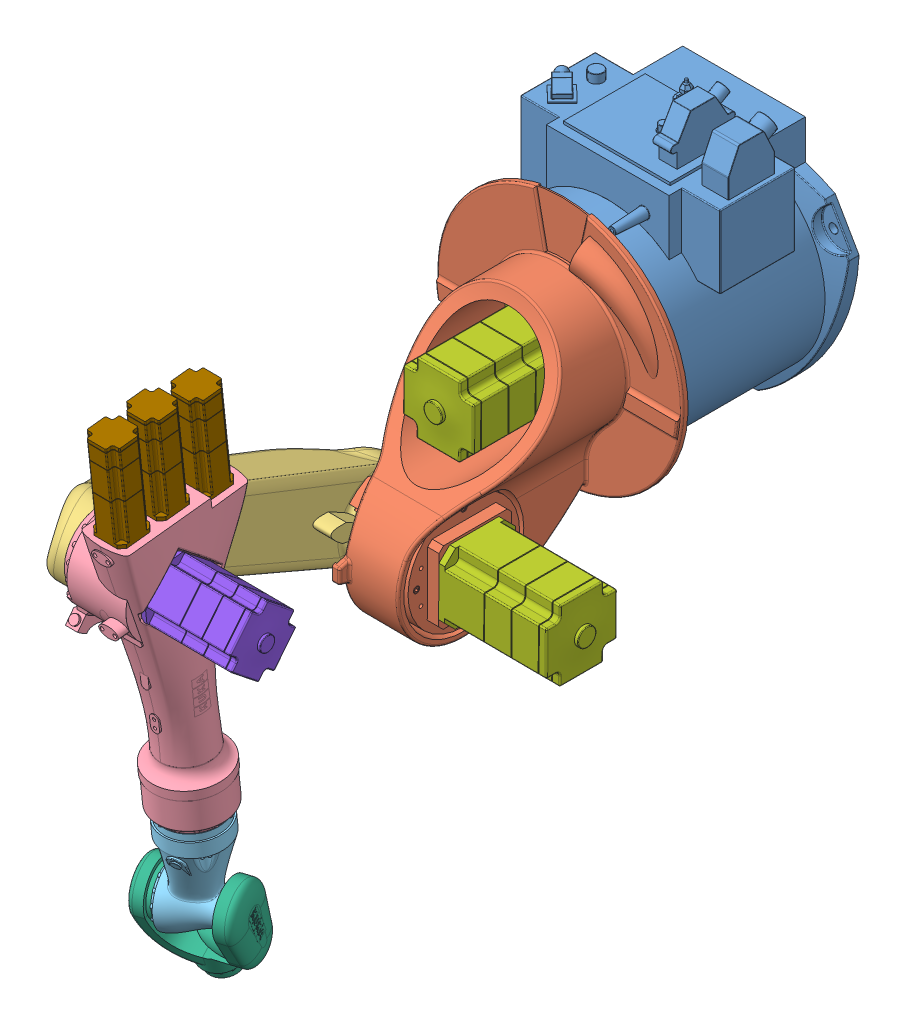
SolidWorks assembly kuka kr16 assembly, configuration Default. Lengths in mm.
Overall size (608.89 1226.23 1449.17).
12 component instances, 9 part files, 32 mates.
Components (placement in the parent):
- base-2: base [Default] at (542.6256 -153.7363 199.462) size (552.23 656.95 396.31)
- rotary head-2: rotary head [Default] at (542.6256 -153.7363 562.462) x (-0.006572 -0.999978 0) z (0 0 1) size (675.15 540 498.16)
- lower arm-2: lower arm [Default] at (425.9194 -412.9749 844.462) x (-0.006078 -0.924775 0.380466) z (-0.999978 0.006572 0) size (217.18 850 204)
- upper arm-2: upper arm [Default] at (557.5213 -626.142 1397.8001) x (-0.006531 -0.993735 -0.111569) z (-0.999978 0.006572 0) size (623.51 290.87 209)
- p2-2: p2 [Default] at (557.5213 -626.142 1397.8001) x (-0.272397 0.10912 -0.955977) z (0.006531 0.993735 0.111569) size (141.25 136.16 254.9)
- WRIST-2: WRIST [Default] at (606.3129 -813.696 1362.4889) x (-0.085206 -0.919446 -0.383875) z (0.962163 0.024148 -0.271403) size (217.6 120.26 202.46)
- a1servo-3: a1servo [Default] at (542.6256 -153.7363 605.462) x (-0.006572 -0.999978 0) z (0 0 1) size (155 155 249)
- a1servo-4: a1servo [Default] at (625.8986 -416.7893 846.962) x (-0.006572 -0.999978 0) z (0.999978 -0.006572 0) size (155 155 249)
- a3servo-2: a3servo [Default] at (573.4266 -155.2216 1473.3224) x (-0.0041 -0.623787 -0.781584) z (0.999978 -0.006572 0) size (126 126 202.41)
- a4a5a6 servo-4: a4a5a6 servo [Default] at (561.5909 -6.9114 1470.5995) x (-0.000733 -0.111567 0.993757) z (0.006531 0.993735 0.111569) size (72 72 200)
- a4a5a6 servo-5: a4a5a6 servo [Default] at (561.527 -16.6375 1557.2324) x (-0.000733 -0.111567 0.993757) z (0.006531 0.993735 0.111569) size (72 72 200)
- a4a5a6 servo-6: a4a5a6 servo [Default] at (561.524 -17.0874 1373.016) x (-0.000733 -0.111567 0.993757) z (0.006531 0.993735 0.111569) size (72 72 200)
Mates (geometry in assembly coordinates):
- Concentric1: concentric aligned: cylinder of base-2 through (542.6256 -153.7363 562.462) axis (0 0 -1) radius 215; cylinder of rotary head-2 through (542.6256 -153.7363 975.462) axis (0 0 -1) radius 120
- Coincident1: coincident anti-aligned: plane of base-2 through (542.6256 -153.7363 562.462) normal (0 0 1); plane of rotary head-2 through (542.6256 -153.7363 562.462) normal (0 0 -1)
- Coincident2: coincident anti-aligned: plane of rotary head-2 through (467.6272 -153.2434 562.462) normal (-0.999978 0.006572 0); plane of lower arm-2 through (466.3345 -349.941 1001.8842) normal (0.999978 -0.006572 0)
- Concentric2: concentric anti-aligned: circle of rotary head-2; cylinder of lower arm-2 through (-44.0705 -409.8861 844.462) axis (0.999978 -0.006572 0) radius 90
- Coincident3: coincident anti-aligned: plane of lower arm-2 through (428.9193 -412.9947 844.462) normal (0.999978 -0.006572 0); plane of upper arm-2 through (430.6196 -154.2831 1473.3224) normal (-0.999978 0.006572 0)
- Coincident4: coincident anti-aligned: circle of lower arm-2; cylinder of upper arm-2 through (453.6191 -154.4342 1473.3224) axis (-0.999978 0.006572 0) radius 80
- Concentric3: concentric aligned: cylinder of upper arm-2 through (559.0727 -390.0862 1424.3027) axis (0.006531 0.993735 0.111569) radius 77; cylinder of p2-2 through (557.2143 -672.8476 1392.5563) axis (0.006531 0.993735 0.111569) radius 67.5
- Coincident5: coincident anti-aligned: plane of upper arm-2 through (557.5213 -626.142 1397.8001) normal (-0.006531 -0.993735 -0.111569); plane of p2-2 through (557.5213 -626.142 1397.8001) normal (0.006531 0.993735 0.111569)
- Coincident6: coincident anti-aligned: plane of p2-2 through (496.6263 -816.4488 1393.4288) normal (-0.962163 -0.024148 0.271403); plane of WRIST-2 through (496.6263 -816.4488 1393.4288) normal (0.962163 0.024148 -0.271403)
- Concentric4: concentric anti-aligned: circle of p2-2; circle of WRIST-2
- Coincident8: coincident anti-aligned: plane of rotary head-2 through (542.6256 -153.7363 605.462) normal (0 0 1); plane of a1servo-3 through (542.6256 -153.7363 605.462) normal (0 0 -1)
- Coincident9: coincident aligned: plane of rotary head-2; plane of a1servo-3
- Coincident10: coincident aligned: plane of rotary head-2; plane of a1servo-3
- Coincident11: coincident anti-aligned: plane of rotary head-2 through (627.6238 -154.295 562.462) normal (0.999978 -0.006572 0); plane of a1servo-4 through (625.8986 -416.7893 846.962) normal (-0.999978 0.006572 0)
- Coincident12: coincident aligned: plane of rotary head-2 through (625.3893 -494.2876 562.462) normal (-0.006572 -0.999978 0); plane of a1servo-4 through (638.389 -494.373 846.962) normal (-0.006572 -0.999978 0)
- Coincident13: coincident: plane of rotary head-2 through (627.6238 -154.295 924.462) normal (0 0 1); line of a1servo-4 through (626.2536 -362.7686 924.462) axis (-0.006572 -0.999978 0)
- Coincident14: coincident aligned: plane of a4a5a6 servo-4; plane of a4a5a6 servo-5
- Coincident15: coincident aligned: plane of a4a5a6 servo-5; plane of a4a5a6 servo-6
- Coincident17: coincident aligned: plane of a4a5a6 servo-4 through (561.5909 -6.9114 1470.5995) normal (0.006531 0.993735 0.111569); plane of a4a5a6 servo-5 through (561.527 -16.6375 1557.2324) normal (0.006531 0.993735 0.111569)
- Coincident18: coincident anti-aligned: plane of upper arm-2 through (557.5213 -626.142 1397.8001) normal (-0.999978 0.006572 0); plane of a4a5a6 servo-5
- Coincident19: coincident anti-aligned: plane of upper arm-2 through (561.7043 10.3459 1316.8846) normal (0.006531 0.993735 0.111569); plane of a4a5a6 servo-4 through (561.5909 -6.9114 1470.5995) normal (-0.006531 -0.993735 -0.111569)
- Coincident20: coincident anti-aligned: plane of upper arm-2 through (561.4562 -27.4166 1465.0206) normal (0.006531 0.993735 0.111569); plane of a4a5a6 servo-6 through (561.524 -17.0874 1373.016) normal (-0.006531 -0.993735 -0.111569)
- Lock2: lock: unknown of upper arm-2; unknown of a4a5a6 servo-5
- Lock3: lock: unknown of upper arm-2; unknown of a4a5a6 servo-4
- Lock4: lock: unknown of upper arm-2; unknown of a4a5a6 servo-6
- Coincident22: coincident anti-aligned: plane of upper arm-2 through (592.5205 -626.372 1397.8001) normal (0.999978 -0.006572 0); plane of a3servo-2 through (595.616 -155.3673 1473.3221) normal (-0.999978 0.006572 0)
- Coincident23: coincident: axis of upper arm-2 through (547.9129 -155.054 1473.3224) axis (-0.999978 0.006572 0); plane of a3servo-2
- Coincident24: coincident: axis of upper arm-2 through (547.9129 -155.054 1473.3224) axis (-0.999978 0.006572 0); plane of a3servo-2
- Parallel1: parallel: line of upper arm-2 through (595.0711 -238.2833 1464.0132) axis (0.005137 0.781567 -0.623801); plane of a3servo-2 through (605.9253 -194.7354 1424.0823) normal (-0.0041 -0.623787 -0.781584)
- LimitAngle2: limit planar angle = 1.961097 rad anti-aligned: plane of lower arm-2; plane of rotary head-2 through (542.6256 -153.7363 562.462) normal (0 0 1)
- LimitAngle3: limit planar angle = 2.072899 rad anti-aligned: plane of lower arm-2; plane of upper arm-2
- LimitAngle4: limit planar angle = 0.294075 rad aligned: plane of WRIST-2; plane of p2-2
